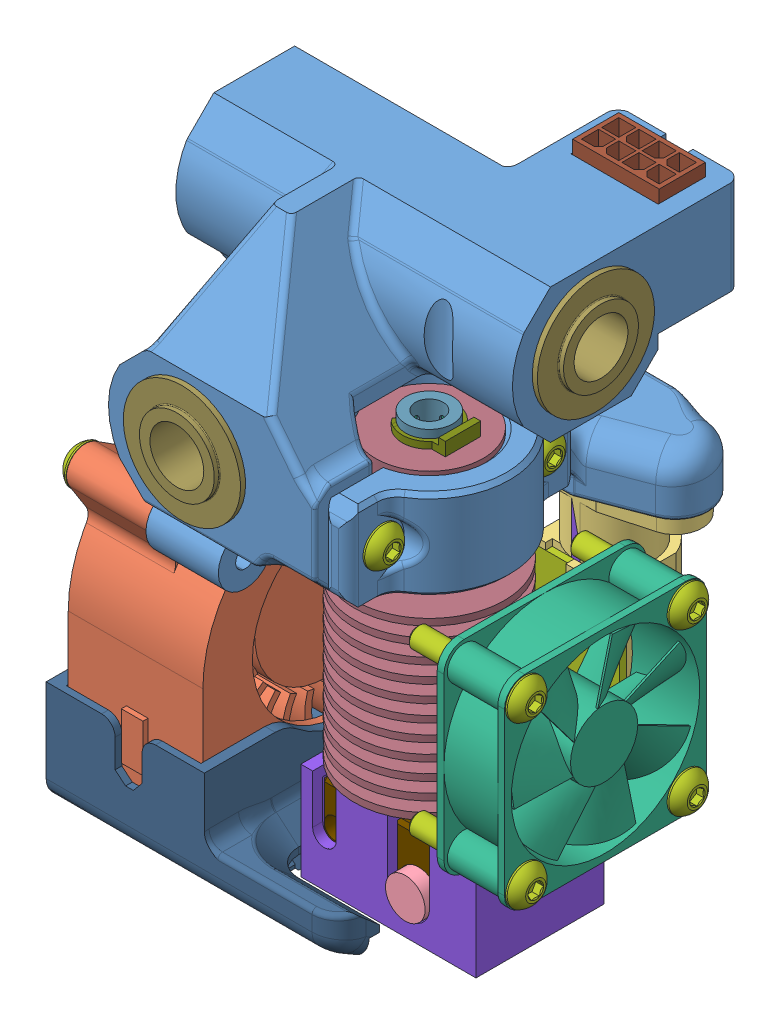
SolidWorks assembly BlTouch_Compact_Carriage_V2.5, configuration Default. Lengths in mm.
Overall size (69.95 84.55 53.81).
51 component instances, 28 part files, 56 mates.
Components (placement in the parent):
- Center Carriage With BLTouch-1: Center Carriage With BLTouch [Default] at (-10.1742 2.5927 -6.0329) size (51.06 40.66 53.16)
- 4020Blower_R3-1: 4020Blower_R3 [Default] at (-18.4242 -34.5229 12.3516) x (0 -1 0) z (0 0 1) size (40.83 20 46.25)
- BLTouch-1: BLTouch [Retracted] at (5.8258 -20.4073 -12.5679) x (-1 0 0) z (0 0 1) size (26 41.3 11.78)
  - Component1-1: Component1 [Default] at origin size (26 36.3 11.78)
  - Pin-1: Pin [Default] at (0 -7.1 0) size (3 34.6 3)
  - Component3-1: Component3 [Default] at (0 -7.1 0) size (3 3.7 3)
  - M4 grub-1: M4 grub [Default] at (9 4.9 0) x (0 1 0) z (0 0 1) size (10 4.01 4.01)
  - BLTouch Classic-1: BLTouch Classic [Default] at origin size (13 20.3 1)
  - BLTouch Classic-0-1: BLTouch Classic-0 [Default] at origin size (1.29 7.7 0)
  - BLTouch Classic-1-1: BLTouch Classic-1 [Default] at origin size (1.29 7.7 0)
- cooling_duct_v2-1: cooling_duct_v2 [Mirror] at (-71.9242 -60.4884 16.6361) x (0 0 1) z (0 1 0) size (44.11 44.53 18)
- 430200801-1: 430200801 [Default] at (0.7458 13.0177 -12.2579) size (14.25 16.89 8.95)
- 2032N24-(8mm Self Align Bronze Sleeve Bearing)-1: 2032N24-(8mm Self Align Bronze Sleeve Bearing) [Default] at (10.5758 9.5927 3.9671) x (0 -0.297233 0.954805) z (0 -0.954805 -0.297233) size (17.4 11.55 17.4)
- 2032N24-(8mm Self Align Bronze Sleeve Bearing)-2: 2032N24-(8mm Self Align Bronze Sleeve Bearing) [Default] at (-20.1742 -4.4073 -16.7829) x (0.954805 -0.297233 0) z (-0.297233 -0.954805 0) size (17.4 11.55 17.4)
- 2032N24-(8mm Self Align Bronze Sleeve Bearing)-4: 2032N24-(8mm Self Align Bronze Sleeve Bearing) [Default] at (-40.9242 9.5927 3.9671) x (0 0.795564 -0.60587) z (0 -0.60587 -0.795564) size (17.4 11.55 17.4)
- 2032N24-(8mm Self Align Bronze Sleeve Bearing)-6: 2032N24-(8mm Self Align Bronze Sleeve Bearing) [Default] at (-20.1742 -4.4073 34.7171) x (-0.219991 -0.975502 0) z (0.975502 -0.219991 0) size (17.4 11.55 17.4)
- e3D V6 1.75mm Hotend Assembly-1: e3D V6 1.75mm Hotend Assembly [Default] at (-1.2453 -61.7573 16.9671) x (-1 0 0) z (0 1 0) size (39.3 30.11 64.51)
  - V6-175-SINK-1: V6-175-SINK [Default] at (-0.0711 0 18.6) x (1 0.000031 0) z (0 0 1) size (22.73 22.73 45.2)
    - V6-175-SINK-1: V6-175-SINK [Default] at origin size (22.73 22.73 43.15)
    - PTFE Tube Retainer-1: PTFE Tube Retainer [Default] at (0 0 1) x (-0.000024 -1 0) z (0 0 1) size (8 9 6.75)
      - Collet-1: Collet [Default] at (0 0 43.9) x (0 1 0) z (0 0 1) size (7 7 6.75)
      - Coupling-1: Coupling [Default] at (0 0 41.7) x (-0.000024 1 0) z (0 0 1) size (8 8 3.48)
      - Collet Clip-1: Collet Clip [Default] at (0 0 41.7) size (8 8.46 2)
  - V6-Heatbreak-1: V6-Heatbreak [Default] at (-0.071 0.0711 11.5) x (-1 -0.000034 0) z (0 0 1) size (6.96 6.95 22.17)
  - V6-Heatblock-1: V6-Heatblock [Default] at (-0.071 0.0711 5) x (1 0.000009 0) z (0 0 1) size (24.18 21 13.72)
    - V6-Heatblock-1: V6-Heatblock [Default] at origin size (23 16.1 11.72)
    - M3x10 rounded head screw - 92095A182 (1)-1: M3x10 rounded head screw - 92095A182 (1) [Default] at (-12.5025 0 -1.6476) x (0.335243 0.942132 0) z (0 0 -1) size (5.74 5.77 12.03)
    - M3x4 flat tip set screw - 92605A098-1: M3x4 flat tip set screw - 92605A098 [Default] at (6.0115 0 2.0029) x (-1 0.000002 0) z (0 0 -1) size (3.04 3.09 4.1)
    - Thermistor-1: Thermistor [Default] at (-0.0065 -2.7408 13.5951) x (1 0 0.000823) z (-0.000823 0 1) size (3 13.5 3)
    - Heater Cartridge-1: Heater Cartridge [Default] at (0.0988 0 0.1652) x (0.999682 0 0.025219) z (-0.025219 0 0.999682) size (5.9 21 5.9)
  - V6-175-Nozzle 0.4mm-1: V6-175-Nozzle 0.4mm [Default] at (-0.071 0.0711 1) x (1 0.000007 0) z (0 0 1) size (8.08 7.02 12.54)
  - Fan Assembly-1: Fan Assembly [Default] at (0 -26 15) size (33.82 30.11 30.05)
    - Fan Shroud-1: Fan Shroud [Default] at (-16.2408 26 3.6) x (0 -1 0) z (0 0 1) size (30.11 22.16 30.05)
    - 30x10mm box fan-1: 30x10mm box fan [Default] at (-26.2408 26 18.6) x (0 -1 0) z (0 0 1) size (30 10.31 30)
    - Trimcraft M3 BSC-5: Trimcraft M3 BSC [3mm x 16mm SST BSC] at (-27.8908 14 6.6) x (0 -1 0) z (-1 0 0) size (5.7 5.7 17.77)
    - Trimcraft M3 BSC-6: Trimcraft M3 BSC [3mm x 16mm SST BSC] at (-27.8908 38 6.6) x (0 0 -1) z (-1 0 0) size (5.7 5.7 17.77)
    - Trimcraft M3 BSC-3: Trimcraft M3 BSC [3mm x 16mm SST BSC] at (-27.8908 38 30.6) x (0 1 0) z (-1 0 0) size (5.7 5.7 17.77)
    - Trimcraft M3 BSC-4: Trimcraft M3 BSC [3mm x 16mm SST BSC] at (-27.8908 14 30.6) x (0 0 1) z (-1 0 0) size (5.7 5.7 17.77)
  - E3D Sock-1: E3D Sock [Default] at (-0.071 0.0711 5) x (-1 -0.000009 0) z (0 0 -1) size (26.02 19.02 16.5)
- 94180A333_HEAT-SET INSERTS FOR PLASTICS-1: 94180A333_HEAT-SET INSERTS FOR PLASTICS [94180A333] at (-1.1742 -7.1573 4.9671) x (0 0.381849 -0.924225) z (0 -0.924225 -0.381849) size (2.91 6.45 5.56)
- 94180A333_HEAT-SET INSERTS FOR PLASTICS-2: 94180A333_HEAT-SET INSERTS FOR PLASTICS [94180A333] at (-1.1742 -7.1573 28.9671) x (0 0.523557 -0.85199) z (0 -0.85199 -0.523557) size (2.91 6.45 5.56)
- 94180A333_HEAT-SET INSERTS FOR PLASTICS-4: 94180A333_HEAT-SET INSERTS FOR PLASTICS [94180A333] at (5.8258 -20.4073 -12.5679) x (0.24496 0 -0.969533) z (-0.969533 0 -0.24496) size (2.91 6.45 5.56)
- 94180A333_HEAT-SET INSERTS FOR PLASTICS-6: 94180A333_HEAT-SET INSERTS FOR PLASTICS [94180A333] at (-12.1742 -20.4073 -12.5679) x (0.046341 0 -0.998926) z (-0.998926 0 -0.046341) size (2.91 6.45 5.56)
- 94180A333_HEAT-SET INSERTS FOR PLASTICS-8: 94180A333_HEAT-SET INSERTS FOR PLASTICS [94180A333] at (-16.9242 -51.9884 -4.1139) x (0 -0.748132 -0.66355) z (0 -0.66355 0.748132) size (2.91 6.45 5.56)
- Trimcraft M3 BSC-1: Trimcraft M3 BSC [3mm x 25mm SST BSC] at (-43.0742 -51.9884 -4.1139) x (0 0 1) z (-1 0 0) size (5.7 5.7 26.77)
- Trimcraft M3 BSC-2: Trimcraft M3 BSC [3mm x 08mm SST BSC] at (-12.1742 -24.3573 -12.5679) x (1 0 0) z (0 -1 0) size (5.7 5.7 9.77)
- Trimcraft M3 BSC-3: Trimcraft M3 BSC [3mm x 08mm SST BSC] at (5.8258 -24.3573 -12.5679) x (1 0 0) z (0 -1 0) size (5.7 5.7 9.77)
- Trimcraft M3 BSC-4: Trimcraft M3 BSC [3mm x 10mm SST BSC] at (5.4758 -7.1573 28.9671) x (0 0 -1) z (1 0 0) size (5.7 5.7 11.77)
- Trimcraft M3 BSC-5: Trimcraft M3 BSC [3mm x 10mm SST BSC] at (5.4758 -7.1573 4.9671) x (0 0.158553 -0.987351) z (1 0 0) size (5.7 5.7 11.77)
- Trimcraft M3 BSC-7: Trimcraft M3 BSC [3mm x 20mm SST BSC] at (-40.0742 -17.0573 30.8171) x (0 0.375683 0.926748) z (-1 0 0) size (5.7 5.7 21.77)
- Trimcraft M3 BSC-8: Trimcraft M3 BSC [3mm x 20mm SST BSC] at (-40.0742 -16.9884 -4.1829) x (0 0 1) z (-1 0 0) size (5.7 5.7 21.77)
Mates (geometry in assembly coordinates):
- Concentric1: concentric: cylinder of Center Carriage With BLTouch-1 through (-16.6742 -17.0573 30.8171) axis (-1 0 0) radius 1.425; cylinder of 4020Blower_R3-1 through (-25.4242 -17.0573 30.8171) axis (-1 0 0) radius 1.75
- Parallel1: parallel: plane of 4020Blower_R3-1 through (-38.4242 -55.0229 33.3516) normal (0 -1 0); plane of Center Carriage With BLTouch-1 through (-22.9242 -12.6073 19.4671) normal (0 -1 0)
- Concentric3: concentric: cylinder of Center Carriage With BLTouch-1 through (-1.1742 -0.4073 16.9671) axis (0 -1 0) radius 6; cylinder of ? through (-1.1742 -7.1573 16.9671) axis (0 -1 0) radius 6
- Coincident2: coincident: plane of Center Carriage With BLTouch-1 through (-1.1742 -10.1573 39.9671) normal (0 -1 0); plane of ? through (-8.1742 -10.1573 16.9671) normal (0 1 0)
- Parallel2: parallel: plane of 4020Blower_R3-1 through (-35.8242 -34.5229 13.3516) normal (-1 0 0); plane of ? through (14.3258 -45.2573 24.9671) normal (1 0 0)
- Distance1: distance = 8.5 mm: plane of ? through (-1.1742 -62.7573 16.9671) normal (0 -1 0); plane of ? through (-3.1742 -54.2573 -12.5679) normal (0 -1 0)
- Coincident6: coincident: plane of Center Carriage With BLTouch-1 through (9.8258 5.5927 -18.3329) normal (0 0 -1); plane of ? through (-7.1742 -54.2573 -18.3329) normal (0 0 -1)
- Coincident7: coincident: plane of Center Carriage With BLTouch-1 through (9.8258 19.5927 33.9671) normal (1 0 0); moEndPointRef_w of ?
- Coincident29: coincident: plane of Center Carriage With BLTouch-1 through (-25.4242 -24.4073 18.9017) normal (-1 0 0); plane of 4020Blower_R3-1 through (-25.4242 -34.5229 12.3516) normal (1 0 0)
- Concentric5: concentric: cylinder of 4020Blower_R3-1 through (-25.4242 -51.9884 -4.1139) axis (-1 0 0) radius 1.75; cylinder of cooling_duct_v2-1 through (-31.6242 -51.9884 -4.1139) axis (-1 0 0) radius 1.35
- Parallel6: parallel: plane of 4020Blower_R3-1 through (-38.4242 -55.0229 33.3516) normal (0 -1 0); plane of cooling_duct_v2-1 through (-6.9242 -60.4884 16.6361) normal (0 -1 0)
- Coincident13: coincident: plane of 4020Blower_R3-1 through (-38.4242 -34.5229 13.3516) normal (-1 0 0); plane of cooling_duct_v2-1 through (-38.4242 -60.4884 16.6361) normal (1 0 0)
- Coincident14: coincident: plane of Center Carriage With BLTouch-1 through (0.7008 -3.331 -15.6829) normal (0 0 1); plane of 430200801-1 through (-5.6742 4.5727 -15.6829) normal (0 0 -1)
- Coincident15: coincident: plane of Center Carriage With BLTouch-1 through (7.1758 0.4514 -12.1829) normal (-1 0 0); plane of 430200801-1 through (7.1758 13.0177 -12.2579) normal (1 0 0)
- Coincident16: coincident: plane of Center Carriage With BLTouch-1 through (0.7008 5.5927 -12.1829) normal (0 -1 0); plane of 430200801-1 through (-3.8442 5.5927 -14.9829) normal (0 1 0)
- Coincident17: coincident: plane of Center Carriage With BLTouch-1 through (-12.1742 -20.4073 -12.5679) normal (0 -1 0); plane of BLTouch-1/Component1-1 through (-3.1742 -20.4073 -12.5679) normal (0 1 0)
- Concentric6: concentric: cylinder of Center Carriage With BLTouch-1 through (5.8258 -13.4073 -12.5679) axis (0 -1 0) radius 2.525; cylinder of BLTouch-1/Component1-1 through (5.8258 -20.4073 -12.5679) axis (0 -1 0) radius 1.6
- Concentric7: concentric: cylinder of Center Carriage With BLTouch-1 through (-12.1742 -13.4073 -12.5679) axis (0 -1 0) radius 2.525; cylinder of BLTouch-1/Component1-1 through (-12.1742 -20.4073 -12.5679) axis (0 -1 0) radius 1.6
- Concentric8: concentric: cylinder of Center Carriage With BLTouch-1 through (-0.1742 9.5927 3.9671) axis (1 0 0) radius 7.975; cylinder of 2032N24-(8mm Self Align Bronze Sleeve Bearing)-1 through (-0.7642 9.5927 3.9671) axis (1 0 0) radius 8.7
- Coincident18: coincident: plane of Center Carriage With BLTouch-1 through (9.8258 19.5927 33.9671) normal (1 0 0); circle of 2032N24-(8mm Self Align Bronze Sleeve Bearing)-1
- Concentric9: concentric: cylinder of Center Carriage With BLTouch-1 through (-20.1742 -4.4073 -6.0329) axis (0 0 -1) radius 7.975; cylinder of 2032N24-(8mm Self Align Bronze Sleeve Bearing)-2 through (-20.1742 -4.4073 -5.4429) axis (0 0 -1) radius 8.7
- Coincident19: coincident: plane of Center Carriage With BLTouch-1 through (-10.1742 2.5927 -16.0329) normal (0 0 -1); circle of 2032N24-(8mm Self Align Bronze Sleeve Bearing)-2
- Concentric10: concentric: cylinder of Center Carriage With BLTouch-1 through (-30.1742 9.5927 3.9671) axis (-1 0 0) radius 7.975; cylinder of 2032N24-(8mm Self Align Bronze Sleeve Bearing)-4 through (-29.5842 9.5927 3.9671) axis (-1 0 0) radius 8.7
- Coincident20: coincident: plane of Center Carriage With BLTouch-1 through (-40.1742 2.5927 -6.0329) normal (-1 0 0); circle of 2032N24-(8mm Self Align Bronze Sleeve Bearing)-4
- Concentric11: concentric: cylinder of Center Carriage With BLTouch-1 through (-20.1742 -4.4073 23.9671) axis (0 0 1) radius 7.975; cylinder of 2032N24-(8mm Self Align Bronze Sleeve Bearing)-6 through (-20.1742 -4.4073 23.3771) axis (0 0 1) radius 8.7
- Coincident21: coincident: plane of Center Carriage With BLTouch-1 through (-10.1742 2.5927 33.9671) normal (0 0 1); circle of 2032N24-(8mm Self Align Bronze Sleeve Bearing)-6
- Concentric12: concentric: cylinder of Center Carriage With BLTouch-1 through (-1.1742 -0.4073 16.9671) axis (0 -1 0) radius 6; cylinder of e3D V6 1.75mm Hotend Assembly-1/V6-175-SINK-1/V6-175-SINK-1 through (-1.1742 -10.1573 16.9671) axis (0 1 0) radius 6
- Coincident22: coincident: plane of Center Carriage With BLTouch-1 through (-1.1742 -10.1573 39.9671) normal (0 -1 0); plane of e3D V6 1.75mm Hotend Assembly-1/V6-175-SINK-1/V6-175-SINK-1 through (-1.1742 -10.1573 16.9671) normal (0 1 0)
- Parallel7: parallel: plane of e3D V6 1.75mm Hotend Assembly-1 through (-1.2453 -61.7573 16.9671) normal (-1 0 0); plane of assembly through (0 0 0) normal (1 0 0)
- Concentric13: concentric: cylinder of Center Carriage With BLTouch-1 through (-9.1742 -7.1573 4.9671) axis (1 0 0) radius 2.35; cylinder of 94180A333_HEAT-SET INSERTS FOR PLASTICS-1 through (-1.1742 -7.1573 4.9671) axis (1 0 0) radius 2.415
- Coincident24: coincident: plane of Center Carriage With BLTouch-1 through (-1.1742 41.0776 -6.0329) normal (1 0 0); plane of 94180A333_HEAT-SET INSERTS FOR PLASTICS-1 through (-1.1742 -7.1573 4.9671) normal (1 0 0)
- Concentric14: concentric: cylinder of Center Carriage With BLTouch-1 through (-9.1742 -7.1573 28.9671) axis (1 0 0) radius 2.35; cylinder of 94180A333_HEAT-SET INSERTS FOR PLASTICS-2 through (-1.1742 -7.1573 28.9671) axis (1 0 0) radius 2.415
- Coincident25: coincident: plane of Center Carriage With BLTouch-1 through (-1.1742 41.0776 -6.0329) normal (1 0 0); plane of 94180A333_HEAT-SET INSERTS FOR PLASTICS-2 through (-1.1742 -7.1573 28.9671) normal (1 0 0)
- Concentric15: concentric: cylinder of Center Carriage With BLTouch-1 through (5.8258 -13.4073 -12.5679) axis (0 -1 0) radius 2.525; cylinder of 94180A333_HEAT-SET INSERTS FOR PLASTICS-4 through (5.8258 -20.4073 -12.5679) axis (0 -1 0) radius 2.415
- Coincident26: coincident: plane of Center Carriage With BLTouch-1 through (-12.1742 -20.4073 -12.5679) normal (0 -1 0); plane of 94180A333_HEAT-SET INSERTS FOR PLASTICS-4 through (5.8258 -20.4073 -12.5679) normal (0 -1 0)
- Concentric16: concentric: cylinder of Center Carriage With BLTouch-1 through (-12.1742 -13.4073 -12.5679) axis (0 -1 0) radius 2.525; cylinder of 94180A333_HEAT-SET INSERTS FOR PLASTICS-6 through (-12.1742 -20.4073 -12.5679) axis (0 -1 0) radius 2.415
- Coincident27: coincident: plane of Center Carriage With BLTouch-1 through (-12.1742 -20.4073 -12.5679) normal (0 -1 0); plane of 94180A333_HEAT-SET INSERTS FOR PLASTICS-6 through (-12.1742 -20.4073 -12.5679) normal (0 -1 0)
- Concentric17: concentric: cylinder of cooling_duct_v2-1 through (3.1033 -51.9884 -4.1139) axis (-1 0 0) radius 2.35; cylinder of 94180A333_HEAT-SET INSERTS FOR PLASTICS-8 through (-16.9242 -51.9884 -4.1139) axis (1 0 0) radius 2.415
- Coincident28: coincident: plane of cooling_duct_v2-1 through (-16.9242 -60.4884 16.6361) normal (1 0 0); plane of 94180A333_HEAT-SET INSERTS FOR PLASTICS-8 through (-16.9242 -51.9884 -4.1139) normal (1 0 0)
- Concentric181: concentric: cylinder of cooling_duct_v2-1 through (-31.6242 -51.9884 -4.1139) axis (-1 0 0) radius 1.35; cylinder of Trimcraft M3 BSC-1 through (-43.0742 -51.9884 -4.1139) axis (-1 0 0) radius 2.85
- Coincident301: coincident: plane of cooling_duct_v2-1 through (-41.4242 -51.9884 -4.1139) normal (-1 0 0); plane of Trimcraft M3 BSC-1 through (-41.4242 -54.8384 -4.1139) normal (1 0 0)
- Concentric191: concentric: cylinder of BLTouch-1/Component1-1 through (-12.1742 -20.4073 -12.5679) axis (0 -1 0) radius 1.6; cylinder of Trimcraft M3 BSC-2 through (-12.1742 -24.3573 -12.5679) axis (0 -1 0) radius 2.85
- Coincident311: coincident: plane of BLTouch-1/Component1-1 through (-3.1742 -22.7073 -12.5679) normal (0 -1 0); plane of Trimcraft M3 BSC-2 through (-12.1742 -22.7073 -15.4179) normal (0 1 0)
- Concentric201: concentric: cylinder of BLTouch-1/Component1-1 through (5.8258 -20.4073 -12.5679) axis (0 -1 0) radius 1.6; cylinder of Trimcraft M3 BSC-3 through (5.8258 -24.3573 -12.5679) axis (0 -1 0) radius 2.85
- Coincident321: coincident: plane of BLTouch-1/Component1-1 through (-3.1742 -22.7073 -12.5679) normal (0 -1 0); plane of Trimcraft M3 BSC-3 through (5.8258 -22.7073 -15.4179) normal (0 1 0)
- Concentric21: concentric: cylinder of Center Carriage With BLTouch-1 through (-5.6997 -7.1573 28.9671) axis (1 0 0) radius 1.6; cylinder of Trimcraft M3 BSC-4 through (-6.1742 -7.1573 28.9671) axis (-1 0 0) radius 1.5
- Coincident33: coincident: plane of Center Carriage With BLTouch-1 through (3.8258 35.3278 -6.0329) normal (1 0 0); plane of Trimcraft M3 BSC-4 through (3.8258 -10.0073 28.9671) normal (-1 0 0)
- Concentric22: concentric: cylinder of Center Carriage With BLTouch-1 through (-5.6997 -7.1573 4.9671) axis (1 0 0) radius 1.6; cylinder of Trimcraft M3 BSC-5 through (-6.1742 -7.1573 4.9671) axis (-1 0 0) radius 1.5
- Coincident34: coincident: plane of Center Carriage With BLTouch-1 through (3.8258 35.3278 -6.0329) normal (1 0 0); plane of Trimcraft M3 BSC-5 through (3.8258 -9.9713 4.5153) normal (-1 0 0)
- Concentric231: concentric: cylinder of 4020Blower_R3-1 through (-25.4242 -17.0573 30.8171) axis (-1 0 0) radius 1.75; cylinder of Trimcraft M3 BSC-7 through (-40.0742 -17.0573 30.8171) axis (-1 0 0) radius 2.85
- Concentric24: concentric: cylinder of Trimcraft M3 BSC-7 through (-13.8742 -17.0573 30.8171) axis (1 0 0) radius 1.5; cylinder of ? through (-38.4242 -17.0573 30.8171) axis (-1 0 0) radius 1.6
- Coincident36: coincident: plane of 4020Blower_R3-1 through (-38.4242 -34.5229 13.3516) normal (-1 0 0); plane of ? through (-38.4242 -17.0573 30.8171) normal (1 0 0)
- Coincident37: coincident: plane of Trimcraft M3 BSC-7 through (-38.8742 -19.8977 31.0516) normal (1 0 0); plane of ? through (-38.8742 -17.0573 30.8171) normal (-1 0 0)
- Coincident38: coincident: plane of 4020Blower_R3-1 through (-38.4242 -34.5229 13.3516) normal (-1 0 0); plane of Trimcraft M3 BSC-7 through (-38.4242 -19.6986 31.8878) normal (1 0 0)
- Concentric251: concentric: cylinder of 4020Blower_R3-1 through (-25.4242 -16.9884 -4.1829) axis (-1 0 0) radius 1.75; cylinder of Trimcraft M3 BSC-8 through (-40.0742 -16.9884 -4.1829) axis (-1 0 0) radius 2.85
- Coincident391: coincident: plane of 4020Blower_R3-1 through (-38.4242 -34.5229 13.3516) normal (-1 0 0); plane of Trimcraft M3 BSC-8 through (-38.4242 -19.8384 -4.1829) normal (1 0 0)
